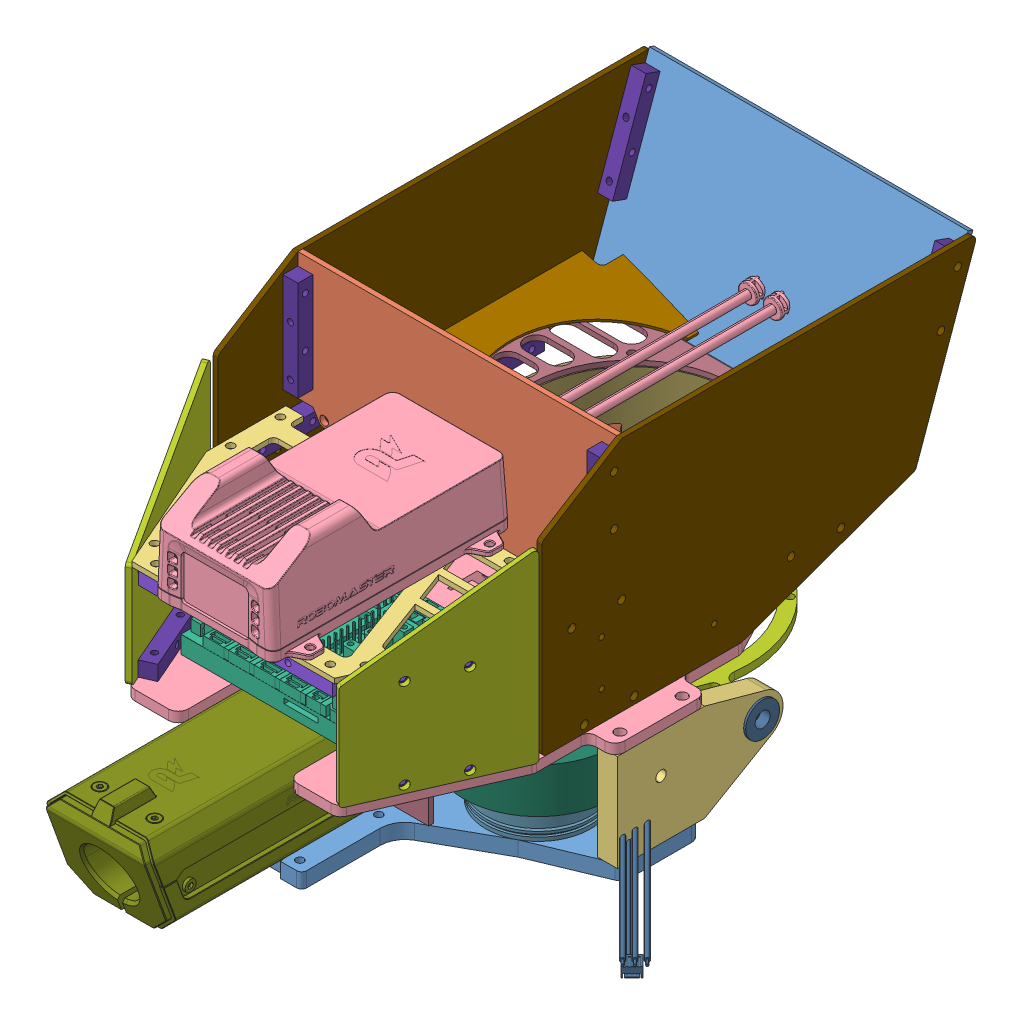
SolidWorks assembly standard robot shooting ver2.0_temp, configuration 默认. Lengths in mm.
Overall size (208.09 148.58 305.3).
60 component instances, 36 part files, 162 mates.
Components (placement in the parent):
- shooting base plate-1: shooting base plate [默认] x (1 0 0) z (0 -1 0) size (153 98.9 6)
- shooting pitch connecting part 01-1: shooting pitch connecting part 01 [默认] at (-76.7 0 8.4) x (0 0 -1) z (1 0 0) size (35 39 8)
- shooting pitch connecting part 02-1: shooting pitch connecting part 02 [默认] at (68.7 0 8.4) x (0 0 -1) z (1 0 0) size (66.5 39 8)
- shooting top plate-1: shooting top plate [默认] at (0 43 -74.1) x (1 0 0) z (0 -1 0) size (153.4 208.1 4)
- bullet tank spacer-1: bullet tank spacer [默认] at (0 34 -74.1) x (-1 0 0) z (0 1 0) size (96 98.1 5)
- bullet tank spacer 02-1: bullet tank spacer 02 [默认] at (0 32.5 -74.1) x (-1 0 0) z (0 1 0) size (96 98.1 1.5)
- bullet tank shell bottom-1: bullet tank shell bottom [默认] at (0 15 -74.1) x (-1 0 0) z (0 1 0) size (94.8 97.5 17.5) (hidden)
- bullet tank base-1: bullet tank base [默认] at (0 12 -74.1) x (-1 0 0) z (0 1 0) size (114 97.1 3)
- barrel end section-1: barrel end section [默认] at (0 23.5 -24) size (48 39 64.7) (hidden)
- bullet feeding motor mounting plate-1: bullet feeding motor mounting plate [默认] at (0 37.9 -74.1) x (0.707107 0 -0.707107) z (0.707107 0 0.707107) size (35 2 35)
- bullet feeding motor mounting part-1: bullet feeding motor mounting part [默认] at (0 13 -74.1) x (0.92388 0 0.382683) z (-0.382683 0 0.92388) size (46 24.9 46)
- RoboMaster M2006 P36-1: RoboMaster M2006 P36 [默认] at (-15.2572 8.0048 -87.7389) x (0 0 -1) z (0 -1 0) size (137.53 138.78 64.81)
- 6mmDshape shaft connector-1: 6mmDshape shaft connector [默认] at (0 43.4 -74.1) x (0.707107 0 -0.707107) z (0 1 0) size (19.05 22 8) (hidden)
- bullet feeding rotor top plate-1: bullet feeding rotor top plate [默认] at (0 51.4 -74.1) x (0.552115 0 0.833768) z (0 1 0) size (64.66 64.66 4) (hidden)
- bullet feeding rotor-1: bullet feeding rotor [默认] at (0 23.9 -74.1) x (0.979638 0 0.20077) z (0 1 0) size (64.66 64.66 27.5)
- bullet tank shell top-1: bullet tank shell top [默认] at (0 66 -74.1) x (1 0 0) z (0 -1 0) size (93.8 93.8 23)
- bullet tank top-1: bullet tank top [默认] at (64 66 -120.5) x (-1 0 0) z (0 1 0) size (128 115 2)
- flywheel-1: flywheel [默认] at (36.5 -8.7 0) x (-0.975794 0 -0.21869) z (0.21869 0 -0.975794) size (75.53 43.7 75.53)
  - M3510 without gearbox-1: M3510 without gearbox [默认] at origin size (42 43.7 47)
  - friction wheel-1: friction wheel [默认] at (0 41.7 0) x (0.951665 0 -0.307138) z (0 -1 0) size (60 60 18)
- flywheel-2: flywheel [默认] at (-36.5 -8.7 0) x (-0.975794 0 -0.21869) z (0.21869 0 -0.975794) size (75.53 43.7 75.53)
  - M3510 without gearbox-1: M3510 without gearbox [默认] at origin size (42 43.7 47)
  - friction wheel-1: friction wheel [默认] at (0 41.7 0) x (0.951665 0 -0.307138) z (0 -1 0) size (60 60 18)
- RM2019 speed detector SM01-1: RM2019 speed detector SM01 [默认] at (21.2957 -30.767 182.229) x (-1 0 0) z (0 0 -1) size (43.41 42.41 109.83)
- plate connector - 4 holes-1: plate connector - 4 holes [默认] at (64 43 -14) x (0 1 0) z (0 0 1) size (6 6 40)
- plate connector - 4 holes-2: plate connector - 4 holes [默认] at (-58 43 -14) x (0 1 0) z (0 0 1) size (6 6 40)
- bullet tank side plate 01-1: bullet tank side plate 01 [默认] at (-64 43 28) x (0 0 1) z (-1 0 0) size (174.16 95 2)
- bullet tank side plate 01-2: bullet tank side plate 01 [默认] at (66 43 28) x (0 0 1) z (-1 0 0) size (174.16 95 2)
- plate connector - 4 holes-3: plate connector - 4 holes [默认] at (-64 135.982 -137.7844) x (0 -0.336336 -0.941742) z (0 -0.941742 0.336336) size (6 6 40)
- plate connector - 4 holes-4: plate connector - 4 holes [默认] at (58 135.982 -137.7844) x (0 -0.336336 -0.941742) z (0 -0.941742 0.336336) size (6 6 40)
- bullet tank side plate 02-1: bullet tank side plate 02 [默认] at (-64 68 -122) x (1 0 0) z (0 0.336336 0.941742) size (128 74.33 2)
- plate connector - 4 holes-5: plate connector - 4 holes [默认] at (-64 133 2) x (0 0 -1) z (0 -1 0) size (6 6 40)
- plate connector - 4 holes-6: plate connector - 4 holes [默认] at (58 133 2) x (0 0 -1) z (0 -1 0) size (6 6 40)
- bullet tank side plate 03-1: bullet tank side plate 03 [默认] at (-64 75 -6) size (128 63 2)
- plate connector - 4 holes-7: plate connector - 4 holes [默认] at (-64 85 -9) x (0 -1 0) z (0 0 1) size (6 6 40)
- plate connector - 4 holes-8: plate connector - 4 holes [默认] at (58 85 -9) x (0 -1 0) z (0 0 1) size (6 6 40)
- camera mounting plate-1: camera mounting plate [默认] at (0 87 -74.1) x (1 0 0) z (0 -1 0) size (127.6 90 2)
- RoboMaster camera VT02 2019 STEP-1: RoboMaster camera VT02 2019 STEP [默认] at (0 91 46) x (-1 0 0) z (0 0 -1) size (60.01 37.51 258.02)
- control board mounting cube-1: control board mounting cube [默认] at (-26 43 41.5) x (0 0 -1) z (0 1 0) size (40 6 6)
- control board mounting cube-2: control board mounting cube [默认] at (38 43 41.5) x (0 0 -1) z (0 1 0) size (40 6 6)
- control board-1: control board [默认] at (-36.5 49 70.5) x (1 0 0) z (0 1 0) size (86 58 17)
- plate connector - 4 holes-9: plate connector - 4 holes [默认] at (-53.5817 43 41.9561) x (0 1 0) z (0.399944 0 0.916539) size (6 6 40)
- plate connector - 4 holes-10: plate connector - 4 holes [默认] at (-53.5817 79 41.9561) x (0 1 0) z (0.399944 0 0.916539) size (6 6 40)
- plate connector - 4 holes-11: plate connector - 4 holes [默认] at (59.081 79 44.3558) x (0 1 0) z (-0.399944 0 0.916539) size (6 6 40)
- plate connector - 4 holes-12: plate connector - 4 holes [默认] at (59.081 43 44.3558) x (0 1 0) z (-0.399944 0 0.916539) size (6 6 40)
- side cover board 01-1: side cover board 01 [默认] at (-42.9165 43 86.3999) x (-0.399944 0 -0.916539) z (0.916539 0 -0.399944) size (61 73.98 2)
- side cover board 01-2: side cover board 01 [默认] at (41.0835 43 85.6001) x (0.399944 0 -0.916539) z (0.916539 0 0.399944) size (61 73.98 2)
- side cover board front connector-1: side cover board front connector [默认] at (39 79 79) x (0 0 1) z (-1 0 0) size (6 6 78)
- side cover board 02-1: side cover board 02 [默认] at (-40 43 85) size (80 42 1) (hidden)
- plate connector - 4 holes-13: plate connector - 4 holes [默认] at (58 66 -97) x (0 -1 0) z (0 0 1) size (6 6 40)
- plate connector - 4 holes-14: plate connector - 4 holes [默认] at (-64 66 -97) x (0 -1 0) z (0 0 1) size (6 6 40)
- plate connector - 4 holes-15: plate connector - 4 holes [默认] at (-57.6096 88.5515 -6) x (-0.233373 -0.972387 0) z (0.972387 -0.233373 0) size (6 6 40)
- plate connector - 4 holes-17: plate connector - 4 holes [默认] at (59.0098 82.7172 -6) x (-0.233373 0.972387 0) z (-0.972387 -0.233373 0) size (6 6 40)
- bullet tank side plate 04-1: bullet tank side plate 04 [默认] at (-20.3477 72.4099 -121) x (-0.972387 0.233373 0) z (0.233373 0.972387 0) size (43 119.07 1)
- bullet tank side plate 04-2: bullet tank side plate 04 [默认] at (20.1143 73.3822 -121) x (0.972387 0.233373 0) z (0.233373 -0.972387 0) size (43 119.07 1)
- bearing flange 12-6-3-1: bearing flange 12-6-3 [默认] at (77.5 23.5 -49.1) x (0 0.841972 0.539522) z (0 -0.539522 0.841972) size (13.6 3.8 13.6)
- bearing flange 12-6-3-2: bearing flange 12-6-3 [默认] at (67.9 23.5 -49.1) x (0 0.977396 -0.211415) z (0 -0.211415 -0.977396) size (13.6 3.8 13.6)
- bullet tank outlet-1: bullet tank outlet [默认] at (24 15 -24) x (-1 0 0) z (0 1 0) size (23.12 18.2 8)
- bullet limits-1: bullet limits [默认] at (0 7 -21.5) x (1 0 0) z (0 1 0) size (27 17.31 11.63)
- barrel end section_U shape design-1: barrel end section_U shape design [默认] at (0 23.5 -24) size (48 43 64.7)
Mates (geometry in assembly coordinates):
- 同心1: concentric aligned: cylinder of shooting base plate-1 through (-72.7 -66.9508 3.4) axis (0 1 0) radius 2.25; cylinder of shooting pitch connecting part 01-1 through (-72.7 0 3.4) axis (0 1 0) radius 1.65
- 同心2: concentric aligned: cylinder of shooting base plate-1 through (-72.7 -66.9508 -21.6) axis (0 1 0) radius 2.25; cylinder of shooting pitch connecting part 01-1 through (-72.7 0 -21.6) axis (0 1 0) radius 1.65
- 重合1: coincident anti-aligned: plane of shooting base plate-1 through (0 0 -36.6787) normal (0 1 0); plane of shooting pitch connecting part 01-1 through (-68.7 0 8.4) normal (0 -1 0)
- 同心3: concentric aligned: cylinder of shooting pitch connecting part 01-1 through (-68.7 23.5 -9.1) axis (-1 0 0) radius 2.1; cylinder of shooting pitch connecting part 02-1 through (76.7 23.5 -9.1) axis (-1 0 0) radius 2.1
- 同心6: concentric anti-aligned: cylinder of shooting pitch connecting part 01-1 through (-72.7 0 -21.6) axis (0 1 0) radius 1.65; cylinder of shooting top plate-1 through (-72.7 81.5161 -21.6) axis (0 -1 0) radius 2.05
- 重合2: coincident anti-aligned: plane of shooting pitch connecting part 01-1 through (-68.7 39 8.4) normal (0 1 0); plane of shooting top plate-1 through (0 39 -74.1) normal (0 -1 0)
- 同心7: concentric anti-aligned: cylinder of shooting top plate-1 through (0 39 -74.1) axis (0 1 0) radius 40.9; cylinder of bullet tank spacer-1 through (0 39 -74.1) axis (0 -1 0) radius 40.9
- 同心8: concentric aligned: cylinder of shooting top plate-1 through (31.7491 39 -105.8491) axis (0 1 0) radius 1.525; cylinder of bullet tank spacer-1 through (31.7491 29 -105.8491) axis (0 1 0) radius 1.525
- 重合3: coincident anti-aligned: plane of shooting top plate-1 through (0 39 -74.1) normal (0 -1 0); plane of bullet tank spacer-1 through (14.2383 39 -26.1702) normal (0 1 0)
- 同心11: concentric aligned: cylinder of bullet tank spacer-1 through (0 39 -74.1) axis (0 -1 0) radius 40.9; cylinder of bullet tank spacer 02-1 through (0 34 -74.1) axis (0 -1 0) radius 40.9
- 同心12: concentric aligned: cylinder of bullet tank spacer-1 through (17.1531 39 -33.6898) axis (0 -1 0) radius 1.525; cylinder of bullet tank spacer 02-1 through (17.1531 34 -33.6898) axis (0 -1 0) radius 1.525
- 重合4: coincident anti-aligned: plane of bullet tank spacer-1 through (14.2383 34 -26.1702) normal (0 -1 0); plane of bullet tank spacer 02-1 through (14.2383 34 -26.1702) normal (0 1 0)
- 同心13: concentric aligned: cylinder of bullet tank spacer-1 through (0 39 -74.1) axis (0 -1 0) radius 40.9; cylinder of bullet tank shell bottom-1 through (0 32.5 -74.1) axis (0 -1 0) radius 40.9
- 同心14: concentric aligned: cylinder of bullet tank spacer-1 through (17.1531 39 -33.6898) axis (0 -1 0) radius 1.525; cylinder of bullet tank shell bottom-1 through (17.1531 32.5 -33.6898) axis (0 -1 0) radius 1.75
- 重合5: coincident anti-aligned: plane of bullet tank spacer 02-1 through (14.2383 32.5 -26.1702) normal (0 -1 0); plane of bullet tank shell bottom-1 through (24 32.5 -24.0021) normal (0 1 0)
- 同心15: concentric aligned: cylinder of bullet tank shell bottom-1 through (0 32.5 -74.1) axis (0 -1 0) radius 40.9; cylinder of bullet tank base-1 through (0 15 -74.1) axis (0 -1 0) radius 17.04
- 同心16: concentric aligned: cylinder of bullet tank shell bottom-1 through (17.1531 32.5 -33.6898) axis (0 -1 0) radius 1.75; cylinder of bullet tank base-1 through (17.1531 15 -33.6898) axis (0 -1 0) radius 1.525
- 重合6: coincident anti-aligned: plane of bullet tank shell bottom-1 through (24 15 -24.0021) normal (0 -1 0); plane of bullet tank base-1 through (14.5654 15 -27.3149) normal (0 1 0)
- 同心17: concentric aligned: cylinder of shooting base plate-1 through (-14 -6 27.5) axis (0 1 0) radius 2.25; cylinder of barrel end section-1 through (-14 0 27.5) axis (0 1 0) radius 2.25
- 同心18: concentric anti-aligned: cylinder of shooting base plate-1 through (0 -6 0) axis (0 1 0) radius 2.25; cylinder of barrel end section-1 through (0 11 0) axis (0 -1 0) radius 1.5
- 重合7: coincident anti-aligned: plane of shooting base plate-1 through (0 0 -36.6787) normal (0 1 0); plane of barrel end section-1 through (25 0 5.7157) normal (0 -1 0)
- 重合8: coincident anti-aligned: plane of bullet tank base-1 through (14.5654 15 -27.3149) normal (0 1 0); plane of bullet feeding motor mounting part-1 through (-15.6136 15 -80.5674) normal (0 -1 0)
- 同心22: concentric aligned: cylinder of bullet tank base-1 through (-7.271 15 -91.6537) axis (0 -1 0) radius 1.525; cylinder of bullet feeding motor mounting part-1 through (-7.271 23 -91.6537) axis (0 -1 0) radius 1.8
- 同心24: concentric aligned: cylinder of bullet feeding motor mounting plate-1 through (-10.4298 37.9 -63.6702) axis (0 1 0) radius 1.3; cylinder of bullet feeding motor mounting part-1 through (-10.4298 13 -63.6702) axis (0 1 0) radius 1.6
- 重合10: coincident anti-aligned: plane of bullet feeding motor mounting plate-1 through (0 37.9 -74.1) normal (0 -1 0); plane of bullet feeding motor mounting part-1 through (-7.3662 37.9 -102.0462) normal (0 1 0)
- 重合11: coincident anti-aligned: plane of bullet feeding motor mounting plate-1 through (0 37.9 -74.1) normal (0 -1 0); plane of RoboMaster M2006 P36-1 through (-8.6267 37.9 -82.7267) normal (0 1 0)
- 同心26: concentric anti-aligned: cylinder of bullet feeding motor mounting plate-1 through (-6.7175 39.9 -80.8175) axis (0 -1 0) radius 1.55; cylinder of RoboMaster M2006 P36-1 through (-6.7175 37.9 -80.8175) axis (0 1 0) radius 1.25
- 同心27: concentric anti-aligned: cylinder of RoboMaster M2006 P36-1 through (0 54.9 -74.1) axis (0 1 0) radius 3; cylinder of 6mmDshape shaft connector-1 through (0 51.4 -74.1) axis (0 -1 0) radius 3
- 重合12: coincident anti-aligned: plane of RoboMaster M2006 P36-1 through (-5.3033 54.9 -72.3322) normal (-0.707107 0 -0.707107); plane of 6mmDshape shaft connector-1 through (-2.9404 51.4 -74.6952) normal (0.707107 0 0.707107)
- 同心28: concentric anti-aligned: cylinder of RoboMaster M2006 P36-1 through (0 54.9 -74.1) axis (0 1 0) radius 3; cylinder of bullet feeding rotor top plate-1 through (0 55.4 -74.1) axis (0 -1 0) radius 3.025
- 重合13: coincident anti-aligned: plane of 6mmDshape shaft connector-1 through (5.6922 51.4 -68.4078) normal (0 1 0); plane of bullet feeding rotor top plate-1 through (31.8144 51.4 -67.6344) normal (0 -1 0)
- 重合14: coincident anti-aligned: plane of RoboMaster M2006 P36-1 through (-5.6569 43.4 -72.6858) normal (0 1 0); plane of 6mmDshape shaft connector-1 through (0 43.4 -74.1) normal (0 -1 0)
- 同心31: concentric aligned: cylinder of bullet feeding motor mounting part-1 through (0 13 -74.1) axis (0 -1 0) radius 17.5; cylinder of bullet feeding rotor-1 through (0 51.4 -74.1) axis (0 -1 0) radius 18.5
- 同心32: concentric anti-aligned: cylinder of bullet feeding rotor top plate-1 through (21.6773 45.4 -77.8544) axis (0 1 0) radius 1.55; cylinder of bullet feeding rotor-1 through (21.6773 51.4 -77.8544) axis (0 -1 0) radius 1.75
- 重合15: coincident anti-aligned: plane of bullet feeding rotor top plate-1 through (31.8144 51.4 -67.6344) normal (0 -1 0); plane of bullet feeding rotor-1 through (27.0975 51.4 -91.9797) normal (0 1 0)
- 同心36: concentric anti-aligned: cylinder of shooting top plate-1 through (31.7491 39 -42.3509) axis (0 1 0) radius 1.525; cylinder of bullet tank shell top-1 through (31.7491 66 -42.3509) axis (0 -1 0) radius 1.75
- 同心37: concentric anti-aligned: cylinder of shooting top plate-1 through (31.7491 39 -105.8491) axis (0 1 0) radius 1.525; cylinder of bullet tank shell top-1 through (31.7491 66 -105.8491) axis (0 -1 0) radius 1.75
- 重合16: coincident anti-aligned: plane of shooting top plate-1 through (0 43 -74.1) normal (0 1 0); plane of bullet tank shell top-1 through (0 43 -74.1) normal (0 -1 0)
- 重合18: coincident anti-aligned: plane of bullet tank shell top-1 through (0 66 -74.1) normal (0 1 0); plane of bullet tank top-1 through (64 66 -120.5) normal (0 -1 0)
- 同心40: concentric aligned: cylinder of bullet tank shell top-1 through (0 43 -74.1) axis (0 1 0) radius 40.9; cylinder of bullet tank top-1 through (0 58 -74.1) axis (0 1 0) radius 41.4
- 同心41: concentric aligned: cylinder of bullet tank shell top-1 through (31.7491 66 -42.3509) axis (0 -1 0) radius 1.75; cylinder of bullet tank top-1 through (31.7491 76 -42.3509) axis (0 -1 0) radius 1.525
- 同心42: concentric aligned: cylinder of shooting base plate-1 through (36.5 -6 0) axis (0 1 0) radius 13.5; cylinder of flywheel-1/M3510 without gearbox-1 through (36.5 35 0) axis (0 1 0) radius 21
- 同心44: concentric anti-aligned: cylinder of shooting base plate-1 through (48.8744 -6 12.3744) axis (0 1 0) radius 1.6; cylinder of flywheel-1/M3510 without gearbox-1 through (48.8744 0 12.3744) axis (0 -1 0) radius 1.65
- 重合19: coincident anti-aligned: plane of shooting base plate-1 through (0 0 -36.6787) normal (0 1 0); plane of flywheel-1/M3510 without gearbox-1 through (23.4244 0 -2.9304) normal (0 -1 0)
- 同心45: concentric aligned: cylinder of shooting base plate-1 through (-36.5 -6 0) axis (0 1 0) radius 13.5; cylinder of flywheel-2/M3510 without gearbox-1 through (-36.5 35 0) axis (0 1 0) radius 21
- 同心46: concentric anti-aligned: cylinder of shooting base plate-1 through (-48.8744 -6 12.3744) axis (0 1 0) radius 1.6; cylinder of flywheel-2/M3510 without gearbox-1 through (-48.8744 0 12.3744) axis (0 -1 0) radius 1.65
- 重合20: coincident anti-aligned: plane of shooting base plate-1 through (0 0 -36.6787) normal (0 1 0); plane of flywheel-2/M3510 without gearbox-1 through (-49.5756 0 -2.9304) normal (0 -1 0)
- 同心47: concentric aligned: cylinder of barrel end section-1 through (0 23.5 -53.6985) axis (0 0 1) radius 10.5; cylinder of RM2019 speed detector SM01-1 through (0 23.5 31.5) axis (0 0 1) radius 10.55
- 同心48: concentric anti-aligned: cylinder of barrel end section-1 through (-24 19.7 37.7) axis (1 0 0) radius 1.75; cylinder of RM2019 speed detector SM01-1 through (-16 19.7 37.7) axis (-1 0 0) radius 1.6
- 同心49: concentric aligned: cylinder of shooting top plate-1 through (61 49 21) axis (0 -1 0) radius 1.55; cylinder of plate connector - 4 holes-1 through (61 93 21) axis (0 -1 0) radius 1.2
- 同心50: concentric aligned: cylinder of shooting top plate-1 through (61 49 1) axis (0 -1 0) radius 1.55; cylinder of plate connector - 4 holes-1 through (61 93 1) axis (0 -1 0) radius 1.2
- 重合21: coincident anti-aligned: plane of shooting top plate-1 through (0 43 -74.1) normal (0 1 0); plane of plate connector - 4 holes-1 through (64 43 26) normal (0 -1 0)
- 同心51: concentric aligned: cylinder of shooting top plate-1 through (-61 49 21) axis (0 -1 0) radius 1.55; cylinder of plate connector - 4 holes-2 through (-61 93 21) axis (0 -1 0) radius 1.2
- 同心52: concentric aligned: cylinder of shooting top plate-1 through (-61 49 1) axis (0 -1 0) radius 1.55; cylinder of plate connector - 4 holes-2 through (-61 93 1) axis (0 -1 0) radius 1.2
- 重合22: coincident anti-aligned: plane of shooting top plate-1 through (0 43 -74.1) normal (0 1 0); plane of plate connector - 4 holes-2 through (-58 43 26) normal (0 -1 0)
- 重合23: coincident anti-aligned: plane of plate connector - 4 holes-2 through (-64 43 26) normal (-1 0 0); plane of bullet tank side plate 01-1 through (-64 43 28) normal (1 0 0)
- 同心53: concentric anti-aligned: cylinder of plate connector - 4 holes-2 through (-14 46 -9) axis (-1 0 0) radius 1.2; cylinder of bullet tank side plate 01-1 through (-66 46 -9) axis (1 0 0) radius 1.6
- 同心54: concentric anti-aligned: cylinder of plate connector - 4 holes-2 through (-14 46 11) axis (-1 0 0) radius 1.2; cylinder of bullet tank side plate 01-1 through (-66 46 11) axis (1 0 0) radius 1.6
- 重合24: coincident anti-aligned: plane of plate connector - 4 holes-1 through (64 43 26) normal (1 0 0); plane of bullet tank side plate 01-2 through (64 43 28) normal (-1 0 0)
- 同心55: concentric anti-aligned: cylinder of plate connector - 4 holes-1 through (108 46 -9) axis (-1 0 0) radius 1.2; cylinder of bullet tank side plate 01-2 through (64 46 -9) axis (1 0 0) radius 1.6
- 同心56: concentric anti-aligned: cylinder of plate connector - 4 holes-1 through (108 46 11) axis (-1 0 0) radius 1.2; cylinder of bullet tank side plate 01-2 through (64 46 11) axis (1 0 0) radius 1.6
- 同心57: concentric aligned: cylinder of bullet tank side plate 01-1 through (-66 130.2643 -138.9279) axis (1 0 0) radius 1.525; cylinder of plate connector - 4 holes-3 through (-108 130.2643 -138.9279) axis (1 0 0) radius 1.2
- 同心58: concentric aligned: cylinder of bullet tank side plate 01-1 through (-66 111.4294 -132.2012) axis (1 0 0) radius 1.525; cylinder of plate connector - 4 holes-3 through (-108 111.4294 -132.2012) axis (1 0 0) radius 1.2
- 重合25: coincident anti-aligned: plane of bullet tank side plate 01-1 through (-64 43 28) normal (1 0 0); plane of plate connector - 4 holes-3 through (-64 98.3123 -124.3309) normal (-1 0 0)
- 同心59: concentric aligned: cylinder of bullet tank side plate 01-2 through (64 130.2643 -138.9279) axis (1 0 0) radius 1.525; cylinder of plate connector - 4 holes-4 through (14 130.2643 -138.9279) axis (1 0 0) radius 1.2
- 同心60: concentric aligned: cylinder of bullet tank side plate 01-2 through (64 111.4294 -132.2012) axis (1 0 0) radius 1.525; cylinder of plate connector - 4 holes-4 through (14 111.4294 -132.2012) axis (1 0 0) radius 1.2
- 重合26: coincident anti-aligned: plane of bullet tank side plate 01-2 through (64 43 28) normal (-1 0 0); plane of plate connector - 4 holes-4 through (64 98.3123 -124.3309) normal (1 0 0)
- 重合27: coincident anti-aligned: plane of plate connector - 4 holes-3 through (-64 96.2943 -129.9814) normal (0 -0.336336 -0.941742); plane of bullet tank side plate 02-1 through (-64 68.6727 -120.1165) normal (0 0.336336 0.941742)
- 同心61: concentric anti-aligned: cylinder of plate connector - 4 holes-3 through (-61 86.2042 -173.0997) axis (0 0.336336 0.941742) radius 1.2; cylinder of bullet tank side plate 02-1 through (-61 101.003 -131.6631) axis (0 -0.336336 -0.941742) radius 1.525
- 同心62: concentric anti-aligned: cylinder of plate connector - 4 holes-4 through (61 105.039 -179.8264) axis (0 0.336336 0.941742) radius 1.2; cylinder of bullet tank side plate 02-1 through (61 119.8378 -138.3898) axis (0 -0.336336 -0.941742) radius 1.525
- 同心63: concentric aligned: cylinder of bullet tank side plate 01-1 through (-66 128 -1) axis (1 0 0) radius 1.525; cylinder of plate connector - 4 holes-5 through (-108 128 -1) axis (1 0 0) radius 1.2
- 同心64: concentric aligned: cylinder of bullet tank side plate 01-1 through (-66 108 -1) axis (1 0 0) radius 1.525; cylinder of plate connector - 4 holes-5 through (-108 108 -1) axis (1 0 0) radius 1.2
- 重合28: coincident anti-aligned: plane of bullet tank side plate 01-1 through (-64 43 28) normal (1 0 0); plane of plate connector - 4 holes-5 through (-64 93 2) normal (-1 0 0)
- 同心65: concentric aligned: cylinder of bullet tank side plate 01-2 through (64 128 -1) axis (1 0 0) radius 1.525; cylinder of plate connector - 4 holes-6 through (14 128 -1) axis (1 0 0) radius 1.2
- 同心66: concentric aligned: cylinder of bullet tank side plate 01-2 through (64 108 -1) axis (1 0 0) radius 1.525; cylinder of plate connector - 4 holes-6 through (14 108 -1) axis (1 0 0) radius 1.2
- 重合30: coincident anti-aligned: plane of bullet tank side plate 01-2 through (64 43 28) normal (-1 0 0); plane of plate connector - 4 holes-6 through (64 93 2) normal (1 0 0)
- 同心67: concentric anti-aligned: cylinder of plate connector - 4 holes-5 through (-61 118 -48) axis (0 0 1) radius 1.2; cylinder of bullet tank side plate 03-1 through (-61 118 -4) axis (0 0 -1) radius 1.75
- 同心68: concentric anti-aligned: cylinder of plate connector - 4 holes-6 through (61 118 -48) axis (0 0 1) radius 1.2; cylinder of bullet tank side plate 03-1 through (61 118 -4) axis (0 0 -1) radius 1.75
- 重合32: coincident anti-aligned: plane of plate connector - 4 holes-5 through (-64 93 -4) normal (0 0 -1); plane of bullet tank side plate 03-1 through (-64 75 -4) normal (0 0 1)
- 同心69: concentric aligned: cylinder of bullet tank side plate 01-1 through (-66 82 16) axis (1 0 0) radius 1.6; cylinder of plate connector - 4 holes-7 through (-108 82 16) axis (1 0 0) radius 1.2
- 同心70: concentric aligned: cylinder of bullet tank side plate 01-1 through (-66 82 -4) axis (1 0 0) radius 1.6; cylinder of plate connector - 4 holes-7 through (-108 82 -4) axis (1 0 0) radius 1.2
- 重合33: coincident anti-aligned: plane of bullet tank side plate 01-1 through (-64 43 28) normal (1 0 0); plane of plate connector - 4 holes-7 through (-64 85 31) normal (-1 0 0)
- 同心71: concentric aligned: cylinder of bullet tank side plate 01-2 through (64 82 16) axis (1 0 0) radius 1.6; cylinder of plate connector - 4 holes-8 through (14 82 16) axis (1 0 0) radius 1.2
- 同心72: concentric aligned: cylinder of bullet tank side plate 01-2 through (64 82 -4) axis (1 0 0) radius 1.6; cylinder of plate connector - 4 holes-8 through (14 82 -4) axis (1 0 0) radius 1.2
- 重合34: coincident anti-aligned: plane of bullet tank side plate 01-2 through (64 43 28) normal (-1 0 0); plane of plate connector - 4 holes-8 through (64 85 31) normal (1 0 0)
- 重合35: coincident anti-aligned: plane of plate connector - 4 holes-7 through (-64 85 31) normal (0 1 0); plane of camera mounting plate-1 through (0 85 -74.1) normal (0 -1 0)
- 同心73: concentric anti-aligned: cylinder of plate connector - 4 holes-8 through (61 35 6) axis (0 1 0) radius 1.2; cylinder of camera mounting plate-1 through (61 95 6) axis (0 -1 0) radius 1.55
- 同心74: concentric anti-aligned: cylinder of plate connector - 4 holes-7 through (-61 35 6) axis (0 1 0) radius 1.2; cylinder of camera mounting plate-1 through (-61 95 6) axis (0 -1 0) radius 1.55
- 同心75: concentric aligned: cylinder of camera mounting plate-1 through (27 77 82) axis (0 1 0) radius 1.3; cylinder of RoboMaster camera VT02 2019 STEP-1 through (27 87 82) axis (0 1 0) radius 1.35
- 同心76: concentric anti-aligned: cylinder of camera mounting plate-1 through (-27 77 82) axis (0 1 0) radius 1.3; cylinder of RoboMaster camera VT02 2019 STEP-1 through (-27 87 82) axis (0 -1 0) radius 1.35
- 重合36: coincident anti-aligned: plane of camera mounting plate-1 through (0 87 -74.1) normal (0 1 0); plane of RoboMaster camera VT02 2019 STEP-1 through (0 87 46) normal (0 -1 0)
- 同心77: concentric anti-aligned: cylinder of shooting top plate-1 through (-26 49 49.5) axis (0 -1 0) radius 1.525; cylinder of control board mounting cube-1 through (-26 43 49.5) axis (0 1 0) radius 1.5
- 同心78: concentric anti-aligned: cylinder of shooting top plate-1 through (-26 49 33.5) axis (0 -1 0) radius 1.525; cylinder of control board mounting cube-1 through (-26 43 33.5) axis (0 1 0) radius 1.5
- 重合37: coincident anti-aligned: plane of shooting top plate-1 through (0 43 -74.1) normal (0 1 0); plane of control board mounting cube-1 through (-26 43 41.5) normal (0 -1 0)
- 同心79: concentric anti-aligned: cylinder of shooting top plate-1 through (38 49 49.5) axis (0 -1 0) radius 1.525; cylinder of control board mounting cube-2 through (38 43 49.5) axis (0 1 0) radius 1.5
- 同心80: concentric anti-aligned: cylinder of shooting top plate-1 through (38 49 33.5) axis (0 -1 0) radius 1.525; cylinder of control board mounting cube-2 through (38 43 33.5) axis (0 1 0) radius 1.5
- 重合38: coincident anti-aligned: plane of shooting top plate-1 through (0 43 -74.1) normal (0 1 0); plane of control board mounting cube-2 through (38 43 41.5) normal (0 -1 0)
- 同心81: concentric anti-aligned: cylinder of control board mounting cube-1 through (-26 43 57.5) axis (0 1 0) radius 1.5; cylinder of control board-1 through (-26 60 57.5) axis (0 -1 0) radius 2.8
- 同心82: concentric anti-aligned: cylinder of control board mounting cube-1 through (-26 43 25.5) axis (0 1 0) radius 1.5; cylinder of control board-1 through (-26 60 25.5) axis (0 -1 0) radius 2.8
- 重合39: coincident anti-aligned: plane of control board mounting cube-1 through (-26 49 41.5) normal (0 1 0); plane of control board-1 through (-36.5 49 70.5) normal (0 -1 0)
- 同心83: concentric aligned: cylinder of shooting top plate-1 through (-50.3322 49 56.904) axis (0 -1 0) radius 1.55; cylinder of plate connector - 4 holes-9 through (-50.3322 93 56.904) axis (0 -1 0) radius 1.2
- 同心85: concentric aligned: cylinder of shooting top plate-1 through (-42.3333 49 75.2348) axis (0 -1 0) radius 1.55; cylinder of plate connector - 4 holes-9 through (-42.3333 93 75.2348) axis (0 -1 0) radius 1.2
- 重合41: coincident anti-aligned: plane of shooting top plate-1 through (0 43 -74.1) normal (0 1 0); plane of plate connector - 4 holes-9 through (-37.5839 43 78.6177) normal (0 -1 0)
- 同心86: concentric aligned: cylinder of camera mounting plate-1 through (-42.3333 95 75.2348) axis (0 -1 0) radius 1.55; cylinder of plate connector - 4 holes-10 through (-42.3333 129 75.2348) axis (0 -1 0) radius 1.2
- 同心87: concentric aligned: cylinder of camera mounting plate-1 through (-50.3322 95 56.904) axis (0 -1 0) radius 1.55; cylinder of plate connector - 4 holes-10 through (-50.3322 129 56.904) axis (0 -1 0) radius 1.2
- 重合42: coincident anti-aligned: plane of camera mounting plate-1 through (0 85 -74.1) normal (0 -1 0); plane of plate connector - 4 holes-10 through (-37.5839 85 78.6177) normal (0 1 0)
- 同心88: concentric aligned: cylinder of camera mounting plate-1 through (42.3333 95 75.2348) axis (0 -1 0) radius 1.55; cylinder of plate connector - 4 holes-11 through (42.3333 129 75.2348) axis (0 -1 0) radius 1.2
- 同心89: concentric aligned: cylinder of camera mounting plate-1 through (50.3322 95 56.904) axis (0 -1 0) radius 1.55; cylinder of plate connector - 4 holes-11 through (50.3322 129 56.904) axis (0 -1 0) radius 1.2
- 重合43: coincident anti-aligned: plane of camera mounting plate-1 through (0 85 -74.1) normal (0 -1 0); plane of plate connector - 4 holes-11 through (43.0832 85 81.0174) normal (0 1 0)
- 同心90: concentric aligned: cylinder of shooting top plate-1 through (42.3333 49 75.2348) axis (0 -1 0) radius 1.55; cylinder of plate connector - 4 holes-12 through (42.3333 93 75.2348) axis (0 -1 0) radius 1.2
- 同心91: concentric aligned: cylinder of shooting top plate-1 through (50.3322 49 56.904) axis (0 -1 0) radius 1.55; cylinder of plate connector - 4 holes-12 through (50.3322 93 56.904) axis (0 -1 0) radius 1.2
- 重合44: coincident anti-aligned: plane of shooting top plate-1 through (0 43 -74.1) normal (0 1 0); plane of plate connector - 4 holes-12 through (43.0832 43 81.0174) normal (0 -1 0)
- 同心93: concentric aligned: cylinder of plate connector - 4 holes-9 through (-11.2543 46 28.9413) axis (-0.916539 0 0.399944) radius 1.2; cylinder of side cover board 01-1 through (-57.0812 46 48.9385) axis (-0.916539 0 0.399944) radius 1.75
- 同心94: concentric aligned: cylinder of plate connector - 4 holes-9 through (-3.2554 46 47.272) axis (-0.916539 0 0.399944) radius 1.2; cylinder of side cover board 01-1 through (-49.0823 46 67.2693) axis (-0.916539 0 0.399944) radius 1.75
- 重合46: coincident anti-aligned: plane of plate connector - 4 holes-9 through (-43.0832 43 81.0174) normal (-0.916539 0 0.399944); plane of side cover board 01-1 through (-41.0835 43 85.6001) normal (0.916539 0 -0.399944)
- 重合47: coincident anti-aligned: plane of plate connector - 4 holes-11 through (43.0832 79 81.0174) normal (0.916539 0 0.399944); plane of side cover board 01-2 through (41.0835 43 85.6001) normal (-0.916539 0 -0.399944)
- 同心95: concentric aligned: cylinder of plate connector - 4 holes-11 through (89.4101 82 84.8668) axis (-0.916539 0 -0.399944) radius 1.2; cylinder of side cover board 01-2 through (50.9154 82 68.0692) axis (-0.916539 0 -0.399944) radius 1.75
- 同心96: concentric aligned: cylinder of plate connector - 4 holes-12 through (97.409 46 66.536) axis (-0.916539 0 -0.399944) radius 1.2; cylinder of side cover board 01-2 through (58.9143 46 49.7384) axis (-0.916539 0 -0.399944) radius 1.75
- 同心97: concentric aligned: cylinder of camera mounting plate-1 through (-35 77 82) axis (0 1 0) radius 1.55; cylinder of side cover board front connector-1 through (-35 5 82) axis (0 1 0) radius 1.2
- 同心98: concentric aligned: cylinder of camera mounting plate-1 through (35 77 82) axis (0 1 0) radius 1.55; cylinder of side cover board front connector-1 through (35 5 82) axis (0 1 0) radius 1.2
- 重合48: coincident anti-aligned: plane of camera mounting plate-1 through (0 85 -74.1) normal (0 -1 0); plane of side cover board front connector-1 through (-39 85 79) normal (0 1 0)
- 同心99: concentric anti-aligned: cylinder of side cover board front connector-1 through (-21 82 5) axis (0 0 1) radius 1.2; cylinder of side cover board 02-1 through (-21 82 86) axis (0 0 -1) radius 1.55
- 同心100: concentric anti-aligned: cylinder of side cover board front connector-1 through (21 82 5) axis (0 0 1) radius 1.2; cylinder of side cover board 02-1 through (21 82 86) axis (0 0 -1) radius 1.55
- 重合49: coincident anti-aligned: plane of side cover board front connector-1 through (-39 79 85) normal (0 0 1); plane of side cover board 02-1 through (-40 43 85) normal (0 0 -1)
- 同心101: concentric anti-aligned: cylinder of bullet tank top-1 through (61 68 -62) axis (0 -1 0) radius 1.525; cylinder of plate connector - 4 holes-13 through (61 16 -62) axis (0 1 0) radius 1.2
- 同心102: concentric anti-aligned: cylinder of bullet tank top-1 through (61 68 -82) axis (0 -1 0) radius 1.525; cylinder of plate connector - 4 holes-13 through (61 16 -82) axis (0 1 0) radius 1.2
- 重合50: coincident anti-aligned: plane of bullet tank top-1 through (64 66 -120.5) normal (0 -1 0); plane of plate connector - 4 holes-13 through (58 66 -57) normal (0 1 0)
- 同心103: concentric anti-aligned: cylinder of bullet tank top-1 through (-61 68 -62) axis (0 -1 0) radius 1.525; cylinder of plate connector - 4 holes-14 through (-61 16 -62) axis (0 1 0) radius 1.2
- 同心104: concentric anti-aligned: cylinder of bullet tank top-1 through (-61 68 -82) axis (0 -1 0) radius 1.525; cylinder of plate connector - 4 holes-14 through (-61 16 -82) axis (0 1 0) radius 1.2
- 重合51: coincident anti-aligned: plane of bullet tank top-1 through (64 66 -120.5) normal (0 -1 0); plane of plate connector - 4 holes-14 through (-64 66 -57) normal (0 1 0)
- 同心105: concentric anti-aligned: cylinder of bullet tank side plate 03-1 through (-53.4477 84.4675 -14) axis (0 0 1) radius 1.75; cylinder of plate connector - 4 holes-15 through (-53.4477 84.4675 38) axis (0 0 -1) radius 1.2
- 同心106: concentric anti-aligned: cylinder of bullet tank side plate 03-1 through (-34 79.8 -14) axis (0 0 1) radius 1.75; cylinder of plate connector - 4 holes-15 through (-34 79.8 38) axis (0 0 -1) radius 1.2
- 重合52: coincident anti-aligned: plane of bullet tank side plate 03-1 through (-64 75 -6) normal (0 0 -1); plane of plate connector - 4 holes-15 through (-18.7141 79.2166 -6) normal (0 0 1)
- 同心107: concentric anti-aligned: cylinder of bullet tank side plate 03-1 through (53.4477 84.4675 -14) axis (0 0 1) radius 1.75; cylinder of plate connector - 4 holes-17 through (53.4477 84.4675 38) axis (0 0 -1) radius 1.2
- 同心108: concentric anti-aligned: cylinder of bullet tank side plate 03-1 through (34 79.8 -14) axis (0 0 1) radius 1.75; cylinder of plate connector - 4 holes-17 through (34 79.8 38) axis (0 0 -1) radius 1.2
- 重合53: coincident anti-aligned: plane of bullet tank side plate 03-1 through (-64 75 -6) normal (0 0 -1); plane of plate connector - 4 holes-17 through (20.1143 73.3822 -6) normal (0 0 1)
- 同心109: concentric anti-aligned: cylinder of plate connector - 4 holes-15 through (-54.6924 36.4315 -9) axis (0.233373 0.972387 0) radius 1.2; cylinder of bullet tank side plate 04-1 through (-44.424 79.2166 -9) axis (-0.233373 -0.972387 0) radius 1.55
- 同心110: concentric anti-aligned: cylinder of plate connector - 4 holes-15 through (-35.2447 31.7641 -9) axis (0.233373 0.972387 0) radius 1.2; cylinder of bullet tank side plate 04-1 through (-24.9762 74.5491 -9) axis (-0.233373 -0.972387 0) radius 1.55
- 重合54: coincident anti-aligned: plane of plate connector - 4 holes-15 through (-20.1143 73.3822 -6) normal (-0.233373 -0.972387 0); plane of bullet tank side plate 04-1 through (-20.1143 73.3822 -121) normal (0.233373 0.972387 0)
- 同心111: concentric anti-aligned: cylinder of plate connector - 4 holes-17 through (32.7553 127.8359 -9) axis (0.233373 -0.972387 0) radius 1.2; cylinder of bullet tank side plate 04-2 through (44.6574 78.2442 -9) axis (-0.233373 0.972387 0) radius 1.55
- 同心112: concentric anti-aligned: cylinder of plate connector - 4 holes-17 through (13.3076 123.1685 -9) axis (0.233373 -0.972387 0) radius 1.2; cylinder of bullet tank side plate 04-2 through (25.2096 73.5767 -9) axis (-0.233373 0.972387 0) radius 1.55
- 重合55: coincident anti-aligned: plane of plate connector - 4 holes-17 through (20.1143 73.3822 -6) normal (0.233373 -0.972387 0); plane of bullet tank side plate 04-2 through (20.1143 73.3822 -121) normal (-0.233373 0.972387 0)
- 同心113: concentric aligned: cylinder of shooting pitch connecting part 02-1 through (18.5677 23.5 -49.1) axis (1 0 0) radius 6; cylinder of bearing flange 12-6-3-1 through (77.5 23.5 -49.1) axis (1 0 0) radius 6
- 重合56: coincident anti-aligned: plane of shooting pitch connecting part 02-1 through (76.7 0 8.4) normal (1 0 0); plane of bearing flange 12-6-3-1 through (76.7 23.5 -49.1) normal (-1 0 0)
- 同心114: concentric anti-aligned: cylinder of shooting pitch connecting part 02-1 through (18.5677 23.5 -49.1) axis (1 0 0) radius 6; cylinder of bearing flange 12-6-3-2 through (67.9 23.5 -49.1) axis (-1 0 0) radius 6
- 重合57: coincident anti-aligned: plane of shooting pitch connecting part 02-1 through (68.7 0 8.4) normal (-1 0 0); plane of bearing flange 12-6-3-2 through (68.7 23.5 -49.1) normal (1 0 0)
- 重合58: coincident anti-aligned: plane of shooting base plate-1 through (0 0 0) normal (0 -1 0); plane of assembly through (0 0 0) normal (0 1 0)
- 重合59: coincident aligned: plane of shooting base plate-1 through (0 0 0) normal (1 0 0); plane of assembly through (0 0 0) normal (1 0 0)
- 重合60: coincident aligned: plane of shooting base plate-1 through (0 0 0) normal (0 0 1); plane of assembly through (0 0 0) normal (0 0 1)
- 同心115: concentric aligned: cylinder of shooting base plate-1 through (72.7 -66.9508 3.4) axis (0 1 0) radius 2.25; cylinder of shooting pitch connecting part 02-1 through (72.7 39 3.4) axis (0 1 0) radius 1.65
- 同心116: concentric aligned: cylinder of bullet feeding motor mounting part-1 through (0 13 -74.1) axis (0 1 0) radius 12.7; cylinder of RoboMaster M2006 P36-1 through (0 54.9 -74.1) axis (0 1 0) radius 12.2
- 同心117: concentric aligned: cylinder of bullet tank base-1 through (0 15 -74.1) axis (0 -1 0) radius 17.04; cylinder of bullet feeding motor mounting part-1 through (0 13 -74.1) axis (0 -1 0) radius 16.9
- 同心118: concentric anti-aligned: cylinder of shooting pitch connecting part 02-1 through (72.7 39 -21.6) axis (0 1 0) radius 1.65; cylinder of shooting top plate-1 through (72.7 81.5161 -21.6) axis (0 -1 0) radius 2.05
- 重合63: coincident anti-aligned: plane of bullet tank base-1 through (14.5654 15 -27.3149) normal (0 1 0); plane of bullet tank outlet-1 through (12 15 -49.05) normal (0 -1 0)
- 同心121: concentric anti-aligned: cylinder of bullet tank base-1 through (-10.5979 7 -38.3339) axis (0 1 0) radius 1.6; cylinder of bullet tank outlet-1 through (-10.5979 23 -38.3339) axis (0 -1 0) radius 1.75
- 同心122: concentric anti-aligned: cylinder of bullet tank base-1 through (-4.8621 7 -46.5254) axis (0 1 0) radius 1.6; cylinder of bullet tank outlet-1 through (-4.8621 23 -46.5254) axis (0 -1 0) radius 1.75
- 重合64: coincident anti-aligned: plane of barrel end section-1 through (-24 8 41) normal (0 -1 0); plane of bullet limits-1 through (3.5 8 -26.5) normal (0 1 0)
- 同心123: concentric aligned: cylinder of barrel end section-1 through (-9.5 15 -21.5) axis (0 -1 0) radius 1.5; cylinder of bullet limits-1 through (-9.5 8 -21.5) axis (0 -1 0) radius 1.6
- 同心124: concentric aligned: cylinder of barrel end section-1 through (9.5 15 -21.5) axis (0 -1 0) radius 1.5; cylinder of bullet limits-1 through (9.5 8 -21.5) axis (0 -1 0) radius 1.6
- 同心125: concentric aligned: cylinder of shooting base plate-1 through (-14 -6 27.5) axis (0 1 0) radius 2.25; cylinder of barrel end section_U shape design-1 through (-14 0 27.5) axis (0 1 0) radius 2.25
- 同心128: concentric aligned: cylinder of shooting base plate-1 through (14 -6 27.5) axis (0 1 0) radius 2.25; cylinder of barrel end section_U shape design-1 through (14 0 27.5) axis (0 1 0) radius 2.25
- 重合65: coincident anti-aligned: plane of shooting base plate-1 through (0 0 -36.6787) normal (0 1 0); plane of barrel end section_U shape design-1 through (25 0 5.7157) normal (0 -1 0)
